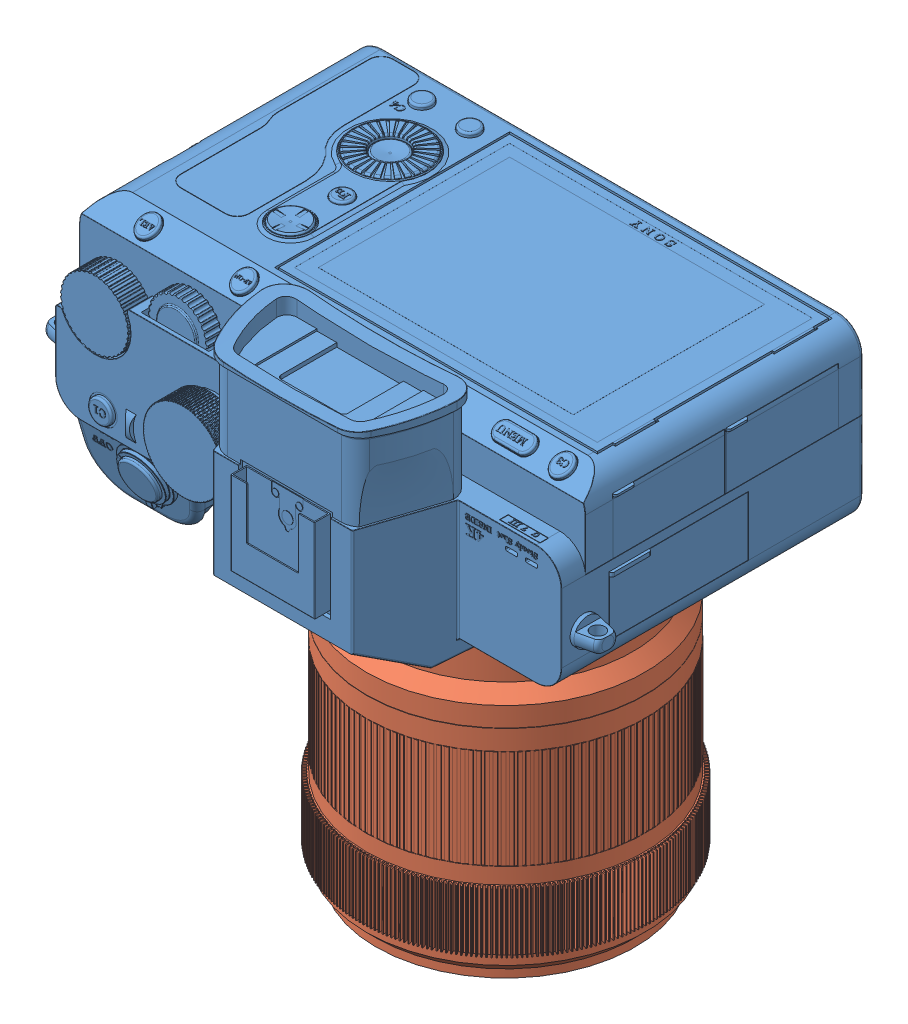
SolidWorks assembly A7 III + FE 28-70 v4, configuration Default. Lengths in mm.
Overall size (139.07 134.7 103.31).
3 component instances, 2 part files, 0 mates.
Components (placement in the parent):
- A7 III + FE 28-70 v4.step-1: A7 III + FE 28-70 v4.step [Default] at origin size (139.07 134.7 103.31)
  - Sony A7 III.step-1: Sony A7 III.step [Default] at origin size (139.07 74.69 103.31)
  - Sony FE 28-70 mm f_3.5-5.6 OSS.step-1: Sony FE 28-70 mm f_3.5-5.6 OSS.step [Default] at (13.5 -93.5 40) size (72.5 83 72.5)
